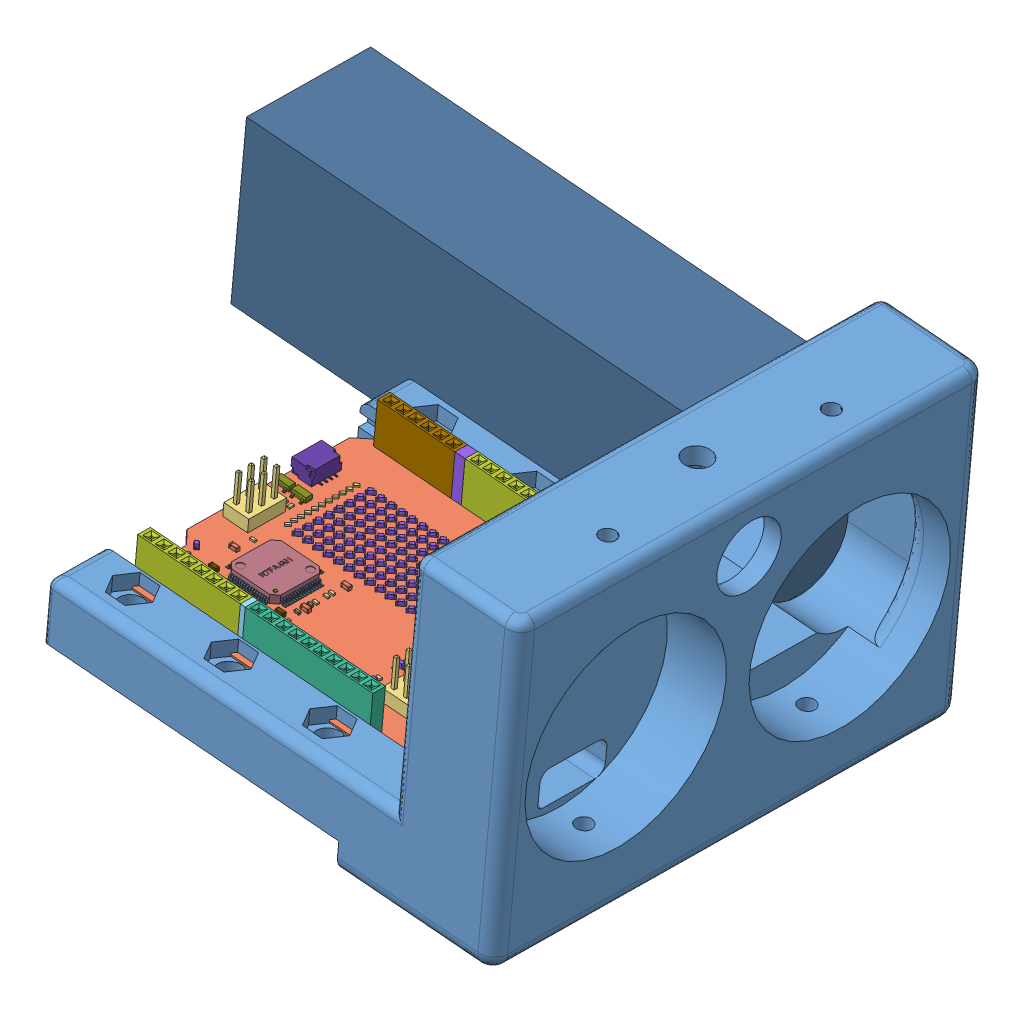
SolidWorks assembly SensorboxController1, configuration Standard. Lengths in mm.
Overall size (130.07 72.74 100.91).
576 component instances, 46 part files, 4 mates.
Components (placement in the parent):
- Sensorbox_small_arduino-1: Sensorbox_small_arduino [Standard] at (44.4865 -57.9317 279.8845) x (0.001937 -0.010295 -0.999945) z (0.996616 -0.082156 0.002776) size (100 64 96.5)
- PCB(ABX00087).step-1: PCB(ABX00087).step [Standard] at (42.9255 -81.7651 134.9822) x (-0.996616 0.082156 -0.002776) z (0.08218 0.996566 -0.010101) size (70.54 53.34 14.5)
  - Board.step-1: Board.step [Standard] at origin size (68.58 53.34 1.61)
    - Open CASCADE STEP translator 7.5 4.1.1.step-1: Open CASCADE STEP translator 7.5 4.1.1.step [Standard] at (0 0 -1.6063) size (68.58 53.34 1.61)
  - R60.step-1: R60.step [Standard] at origin size (1 0.5 0.34)
    - RES-0402.step-1: RES-0402.step [Standard] at (26.4 44.3 0) size (1 0.5 0.34)
  - R59.step-1: R59.step [Standard] at origin size (1 0.5 0.34)
    - RES-0402.step-1: RES-0402.step [Standard] at (26.416 41.021 0) x (-1 0 0) z (0 0 1) size (1 0.5 0.34)
  - R20.step-1: R20.step [Standard] at origin size (1 0.5 0.34)
    - RES-0402.step-1: RES-0402.step [Standard] at (24.29 35.433 0) x (-1 0 0) z (0 0 1) size (1 0.5 0.34)
  - U5.step-1: U5.step [Standard] at origin size (6.71 7 1.8)
    - 6430901664.step-1: 6430901664.step [Standard] at (26.325 10.206 0) x (0 -1 0) z (0 0 1) size (7 6.71 1.8)
      - Body.step-1: Body.step [Standard] at (-1.85 -3.35 0.02) size (3.71 6.71 1.78)
        - Open CASCADE STEP translator 6.8 29.1.1.step-1: Open CASCADE STEP translator 6.8 29.1.1.step [Standard] at origin size (3.71 6.71 1.78)
      - Lead.step-1: Lead.step [Standard] at (-1.85 -2.3 0) x (-1 0 0) z (0 0 1) size (1.65 0.75 1.01)
      - Lead.step-2: Lead.step [Standard] at (-1.85 0 0) x (-1 0 0) z (0 0 1) size (1.65 0.75 1.01)
      - Lead.step-3: Lead.step [Standard] at (-1.85 2.3 0) x (-1 0 0) z (0 0 1) size (1.65 0.75 1.01)
      - Tab.step-1: Tab.step [Standard] at (1.85 0 0) size (1.65 3 1.01)
  - C28.step-1: C28.step [Standard] at origin size (1.25 2 1.25)
    - CAP-0805.step-1: CAP-0805.step [Standard] at (31.0249 12.3561 0) x (0 1 0) z (0 0 1) size (2 1.25 1.25)
  - R58.step-1: R58.step [Standard] at origin size (1 0.5 0.34)
    - RES-0402.step-1: RES-0402.step [Standard] at (16.825 30.966 0) x (-1 0 0) z (0 0 1) size (1 0.5 0.34)
  - R57.step-1: R57.step [Standard] at origin size (1 0.5 0.34)
    - RES-0402.step-1: RES-0402.step [Standard] at (3.625 31.766 0) size (1 0.5 0.34)
  - R16.step-1: R16.step [Standard] at origin size (1.06 1.06 0.34)
    - RES-0402.step-1: RES-0402.step [Standard] at (60.0141 13.5803 0) x (0.707107 0.707107 0) z (0 0 1) size (1 0.5 0.34)
  - R14.step-1: R14.step [Standard] at origin size (1.06 1.06 0.34)
    - RES-0402.step-1: RES-0402.step [Standard] at (60.0141 12.1803 0) x (0.707107 0.707107 0) z (0 0 1) size (1 0.5 0.34)
  - R2.step-1: R2.step [Standard] at origin size (1.06 1.06 0.34)
    - RES-0402.step-1: RES-0402.step [Standard] at (59.9205 26.112 0) x (0.707107 0.707107 0) z (0 0 1) size (1 0.5 0.34)
  - 96.step-1: 96.step [Standard] at origin size (1.7 1.7 0.8)
    - HSMx-190.step-1: HSMx-190.step [Standard] at (57.5124 11.8305 0) x (-0.707107 -0.707107 0) z (0 0 1) size (1.6 0.8 0.8)
  - 95.step-1: 95.step [Standard] at origin size (1.7 1.7 0.8)
    - HSMx-190.step-1: HSMx-190.step [Standard] at (55.4124 11.8305 0) x (-0.707107 -0.707107 0) z (0 0 1) size (1.6 0.8 0.8)
  - 94.step-1: 94.step [Standard] at origin size (1.7 1.7 0.8)
    - HSMx-190.step-1: HSMx-190.step [Standard] at (53.3124 11.8305 0) x (-0.707107 -0.707107 0) z (0 0 1) size (1.6 0.8 0.8)
  - 93.step-1: 93.step [Standard] at origin size (1.7 1.7 0.8)
    - HSMx-190.step-1: HSMx-190.step [Standard] at (51.2124 11.8305 0) x (-0.707107 -0.707107 0) z (0 0 1) size (1.6 0.8 0.8)
  - 92.step-1: 92.step [Standard] at origin size (1.7 1.7 0.8)
    - HSMx-190.step-1: HSMx-190.step [Standard] at (49.1124 11.8305 0) x (-0.707107 -0.707107 0) z (0 0 1) size (1.6 0.8 0.8)
  - 91.step-1: 91.step [Standard] at origin size (1.7 1.7 0.8)
    - HSMx-190.step-1: HSMx-190.step [Standard] at (47.0124 11.8305 0) x (-0.707107 -0.707107 0) z (0 0 1) size (1.6 0.8 0.8)
  - 90.step-1: 90.step [Standard] at origin size (1.7 1.7 0.8)
    - HSMx-190.step-1: HSMx-190.step [Standard] at (44.9124 11.8305 0) x (-0.707107 -0.707107 0) z (0 0 1) size (1.6 0.8 0.8)
  - 89.step-1: 89.step [Standard] at origin size (1.7 1.7 0.8)
    - HSMx-190.step-1: HSMx-190.step [Standard] at (42.8124 11.8305 0) x (-0.707107 -0.707107 0) z (0 0 1) size (1.6 0.8 0.8)
  - 88.step-1: 88.step [Standard] at origin size (1.7 1.7 0.8)
    - HSMx-190.step-1: HSMx-190.step [Standard] at (40.7124 11.8305 0) x (-0.707107 -0.707107 0) z (0 0 1) size (1.6 0.8 0.8)
  - 87.step-1: 87.step [Standard] at origin size (1.7 1.7 0.8)
    - HSMx-190.step-1: HSMx-190.step [Standard] at (38.6124 11.8305 0) x (-0.707107 -0.707107 0) z (0 0 1) size (1.6 0.8 0.8)
  - 86.step-1: 86.step [Standard] at origin size (1.7 1.7 0.8)
    - HSMx-190.step-1: HSMx-190.step [Standard] at (36.5124 11.8305 0) x (-0.707107 -0.707107 0) z (0 0 1) size (1.6 0.8 0.8)
  - 85.step-1: 85.step [Standard] at origin size (1.7 1.7 0.8)
    - HSMx-190.step-1: HSMx-190.step [Standard] at (34.4124 11.8305 0) x (-0.707107 -0.707107 0) z (0 0 1) size (1.6 0.8 0.8)
  - 84.step-1: 84.step [Standard] at origin size (1.7 1.7 0.8)
    - HSMx-190.step-1: HSMx-190.step [Standard] at (57.5124 13.9305 0) x (-0.707107 -0.707107 0) z (0 0 1) size (1.6 0.8 0.8)
  - 83.step-1: 83.step [Standard] at origin size (1.7 1.7 0.8)
    - HSMx-190.step-1: HSMx-190.step [Standard] at (55.4124 13.9305 0) x (-0.707107 -0.707107 0) z (0 0 1) size (1.6 0.8 0.8)
  - 82.step-1: 82.step [Standard] at origin size (1.7 1.7 0.8)
    - HSMx-190.step-1: HSMx-190.step [Standard] at (53.3 13.9182 0) x (-0.707107 -0.707107 0) z (0 0 1) size (1.6 0.8 0.8)
  - 81.step-1: 81.step [Standard] at origin size (1.7 1.7 0.8)
    - HSMx-190.step-1: HSMx-190.step [Standard] at (51.2124 13.9305 0) x (-0.707107 -0.707107 0) z (0 0 1) size (1.6 0.8 0.8)
  - 80.step-1: 80.step [Standard] at origin size (1.7 1.7 0.8)
    - HSMx-190.step-1: HSMx-190.step [Standard] at (49.1124 13.9305 0) x (-0.707107 -0.707107 0) z (0 0 1) size (1.6 0.8 0.8)
  - 79.step-1: 79.step [Standard] at origin size (1.7 1.7 0.8)
    - HSMx-190.step-1: HSMx-190.step [Standard] at (47.0124 13.9305 0) x (-0.707107 -0.707107 0) z (0 0 1) size (1.6 0.8 0.8)
  - 78.step-1: 78.step [Standard] at origin size (1.7 1.7 0.8)
    - HSMx-190.step-1: HSMx-190.step [Standard] at (44.9124 13.9305 0) x (-0.707107 -0.707107 0) z (0 0 1) size (1.6 0.8 0.8)
  - 77.step-1: 77.step [Standard] at origin size (1.7 1.7 0.8)
    - HSMx-190.step-1: HSMx-190.step [Standard] at (42.8124 13.9305 0) x (-0.707107 -0.707107 0) z (0 0 1) size (1.6 0.8 0.8)
  - 76.step-1: 76.step [Standard] at origin size (1.7 1.7 0.8)
    - HSMx-190.step-1: HSMx-190.step [Standard] at (40.7124 13.9305 0) x (-0.707107 -0.707107 0) z (0 0 1) size (1.6 0.8 0.8)
  - 75.step-1: 75.step [Standard] at origin size (1.7 1.7 0.8)
    - HSMx-190.step-1: HSMx-190.step [Standard] at (38.6124 13.9305 0) x (-0.707107 -0.707107 0) z (0 0 1) size (1.6 0.8 0.8)
  - 74.step-1: 74.step [Standard] at origin size (1.7 1.7 0.8)
    - HSMx-190.step-1: HSMx-190.step [Standard] at (36.5124 13.9305 0) x (-0.707107 -0.707107 0) z (0 0 1) size (1.6 0.8 0.8)
  - 73.step-1: 73.step [Standard] at origin size (1.7 1.7 0.8)
    - HSMx-190.step-1: HSMx-190.step [Standard] at (34.4124 13.9305 0) x (-0.707107 -0.707107 0) z (0 0 1) size (1.6 0.8 0.8)
  - 72.step-1: 72.step [Standard] at origin size (1.7 1.7 0.8)
    - HSMx-190.step-1: HSMx-190.step [Standard] at (57.5124 16.0305 0) x (-0.707107 -0.707107 0) z (0 0 1) size (1.6 0.8 0.8)
  - 71.step-1: 71.step [Standard] at origin size (1.7 1.7 0.8)
    - HSMx-190.step-1: HSMx-190.step [Standard] at (55.4124 16.0305 0) x (-0.707107 -0.707107 0) z (0 0 1) size (1.6 0.8 0.8)
  - 70.step-1: 70.step [Standard] at origin size (1.7 1.7 0.8)
    - HSMx-190.step-1: HSMx-190.step [Standard] at (53.3124 16.0305 0) x (-0.707107 -0.707107 0) z (0 0 1) size (1.6 0.8 0.8)
  - 69.step-1: 69.step [Standard] at origin size (1.7 1.7 0.8)
    - HSMx-190.step-1: HSMx-190.step [Standard] at (51.2124 16.0305 0) x (-0.707107 -0.707107 0) z (0 0 1) size (1.6 0.8 0.8)
  - 68.step-1: 68.step [Standard] at origin size (1.7 1.7 0.8)
    - HSMx-190.step-1: HSMx-190.step [Standard] at (49.1124 16.0305 0) x (-0.707107 -0.707107 0) z (0 0 1) size (1.6 0.8 0.8)
  - 67.step-1: 67.step [Standard] at origin size (1.7 1.7 0.8)
    - HSMx-190.step-1: HSMx-190.step [Standard] at (47.0124 16.0305 0) x (-0.707107 -0.707107 0) z (0 0 1) size (1.6 0.8 0.8)
  - 66.step-1: 66.step [Standard] at origin size (1.7 1.7 0.8)
    - HSMx-190.step-1: HSMx-190.step [Standard] at (44.9124 16.0305 0) x (-0.707107 -0.707107 0) z (0 0 1) size (1.6 0.8 0.8)
  - 65.step-1: 65.step [Standard] at origin size (1.7 1.7 0.8)
    - HSMx-190.step-1: HSMx-190.step [Standard] at (42.8124 16.0305 0) x (-0.707107 -0.707107 0) z (0 0 1) size (1.6 0.8 0.8)
  - 64.step-1: 64.step [Standard] at origin size (1.7 1.7 0.8)
    - HSMx-190.step-1: HSMx-190.step [Standard] at (40.7124 16.0305 0) x (-0.707107 -0.707107 0) z (0 0 1) size (1.6 0.8 0.8)
  - 63.step-1: 63.step [Standard] at origin size (1.7 1.7 0.8)
    - HSMx-190.step-1: HSMx-190.step [Standard] at (38.6124 16.0305 0) x (-0.707107 -0.707107 0) z (0 0 1) size (1.6 0.8 0.8)
  - 62.step-1: 62.step [Standard] at origin size (1.7 1.7 0.8)
    - HSMx-190.step-1: HSMx-190.step [Standard] at (36.5124 16.0305 0) x (-0.707107 -0.707107 0) z (0 0 1) size (1.6 0.8 0.8)
  - 61.step-1: 61.step [Standard] at origin size (1.7 1.7 0.8)
    - HSMx-190.step-1: HSMx-190.step [Standard] at (34.412 16.0302 0) x (-0.707107 -0.707107 0) z (0 0 1) size (1.6 0.8 0.8)
  - 60.step-1: 60.step [Standard] at origin size (1.7 1.7 0.8)
    - HSMx-190.step-1: HSMx-190.step [Standard] at (57.5124 18.1305 0) x (-0.707107 -0.707107 0) z (0 0 1) size (1.6 0.8 0.8)
  - 59.step-1: 59.step [Standard] at origin size (1.7 1.7 0.8)
    - HSMx-190.step-1: HSMx-190.step [Standard] at (55.4124 18.1305 0) x (-0.707107 -0.707107 0) z (0 0 1) size (1.6 0.8 0.8)
  - 58.step-1: 58.step [Standard] at origin size (1.7 1.7 0.8)
    - HSMx-190.step-1: HSMx-190.step [Standard] at (53.3124 18.1305 0) x (-0.707107 -0.707107 0) z (0 0 1) size (1.6 0.8 0.8)
  - 57.step-1: 57.step [Standard] at origin size (1.7 1.7 0.8)
    - HSMx-190.step-1: HSMx-190.step [Standard] at (51.2124 18.1305 0) x (-0.707107 -0.707107 0) z (0 0 1) size (1.6 0.8 0.8)
  - 56.step-1: 56.step [Standard] at origin size (1.7 1.7 0.8)
    - HSMx-190.step-1: HSMx-190.step [Standard] at (49.1124 18.1305 0) x (-0.707107 -0.707107 0) z (0 0 1) size (1.6 0.8 0.8)
  - U6.step-1: U6.step [Standard] at origin size (2.1 2.21 1.1)
    - 6430901184.step-1: 6430901184.step [Standard] at (12.525 36.466 0) x (-1 0 0) z (0 0 1) size (2.1 2.21 1.1)
      - Body-1.step-1: Body-1.step [Standard] at (-0.7 -1.1 0) size (1.41 2.21 1.1)
        - Open CASCADE STEP translator 7.5 28.2.1.step-1: Open CASCADE STEP translator 7.5 28.2.1.step [Standard] at origin size (1.41 2.21 1.1)
      - Open CASCADE STEP translator 7.5 28.1.step-1: Open CASCADE STEP translator 7.5 28.1.step [Standard] at (-0.7 -1.1 0.001) size (0.18 0.18 0)
      - Leader.step-1: Leader.step [Standard] at (-0.7 -0.65 0) x (-1 0 0) z (0 0 1) size (0.37 0.2 0.6)
      - Leader.step-2: Leader.step [Standard] at (-0.7 0 0) x (-1 0 0) z (0 0 1) size (0.37 0.2 0.6)
      - Leader.step-3: Leader.step [Standard] at (-0.7 0.65 0) x (-1 0 0) z (0 0 1) size (0.37 0.2 0.6)
      - Leader.step-4: Leader.step [Standard] at (0.7 -0.65 0) size (0.37 0.2 0.6)
      - Leader.step-5: Leader.step [Standard] at (0.7 0 0) size (0.37 0.2 0.6)
      - Leader.step-6: Leader.step [Standard] at (0.7 0.65 0) size (0.37 0.2 0.6)
  - U2.step-1: U2.step [Standard] at origin size (2.1 2.21 1.1)
    - 6430901184.step-1: 6430901184.step [Standard] at (12.525 39.266 0) x (-1 0 0) z (0 0 1) size (2.1 2.21 1.1)
      - Body-1.step-1: Body-1.step [Standard] at (-0.7 -1.1 0) size (1.41 2.21 1.1)
        - Open CASCADE STEP translator 7.5 28.2.1.step-1: Open CASCADE STEP translator 7.5 28.2.1.step [Standard] at origin size (1.41 2.21 1.1)
      - Open CASCADE STEP translator 7.5 28.1.step-1: Open CASCADE STEP translator 7.5 28.1.step [Standard] at (-0.7 -1.1 0.001) size (0.18 0.18 0)
      - Leader.step-1: Leader.step [Standard] at (-0.7 -0.65 0) x (-1 0 0) z (0 0 1) size (0.37 0.2 0.6)
      - Leader.step-2: Leader.step [Standard] at (-0.7 0 0) x (-1 0 0) z (0 0 1) size (0.37 0.2 0.6)
      - Leader.step-3: Leader.step [Standard] at (-0.7 0.65 0) x (-1 0 0) z (0 0 1) size (0.37 0.2 0.6)
      - Leader.step-4: Leader.step [Standard] at (0.7 -0.65 0) size (0.37 0.2 0.6)
      - Leader.step-5: Leader.step [Standard] at (0.7 0 0) size (0.37 0.2 0.6)
      - Leader.step-6: Leader.step [Standard] at (0.7 0.65 0) size (0.37 0.2 0.6)
  - C30.step-1: C30.step [Standard] at origin size (1 0.5 0.5)
    - CAP-0402.step-1: CAP-0402.step [Standard] at (12.525 41.266 0) x (-1 0 0) z (0 0 1) size (1 0.5 0.5)
  - C29.step-1: C29.step [Standard] at origin size (0.5 1 0.5)
    - CAP-0402.step-1: CAP-0402.step [Standard] at (11.925 34.231 0) x (0 1 0) z (0 0 1) size (1 0.5 0.5)
  - R3.step-1: R3.step [Standard] at origin size (0.5 1 0.34)
    - RES-0402.step-1: RES-0402.step [Standard] at (13.466 47.244 0) x (0 -1 0) z (0 0 1) size (1 0.5 0.34)
  - M1.step-1: M1.step [Standard] at origin size (20.65 15.55 2.45)
    - 6428909520.step-1: 6428909520.step [Standard] at (13.625 21.5 0.05) size (13.55 14.15 2.45)
      - Extruded.step-1: Extruded.step [Standard] at origin size (13.55 14.15 2.45)
    - 6428905200.step-1: 6428905200.step [Standard] at (10.575 21.5 0.05) size (20.65 15.55 0.8)
      - Extruded-0.step-1: Extruded-0.step [Standard] at origin size (20.65 15.55 0.8)
  - F1.step-1: F1.step [Standard] at origin size (3.4 4.8 1.4)
    - 6431039776.step-1: 6431039776.step [Standard] at (9.125 32.603 0) size (3.4 4.8 1.4)
      - Extruded-1.step-1: Extruded-1.step [Standard] at origin size (3.4 4.8 1.4)
  - R52.step-1: R52.step [Standard] at origin size (1 0.5 0.34)
    - RES-0402.step-1: RES-0402.step [Standard] at (9.125 42.8599 0) size (1 0.5 0.34)
  - R26.step-1: R26.step [Standard] at origin size (1 0.5 0.34)
    - RES-0402.step-1: RES-0402.step [Standard] at (6.025 30.666 0) x (-1 0 0) z (0 0 1) size (1 0.5 0.34)
  - R12.step-1: R12.step [Standard] at origin size (0.5 1 0.34)
    - RES-0402.step-1: RES-0402.step [Standard] at (67.2698 22.8345 0) x (0 -1 0) z (0 0 1) size (1 0.5 0.34)
  - R11.step-1: R11.step [Standard] at origin size (0.5 1 0.34)
    - RES-0402.step-1: RES-0402.step [Standard] at (66.0698 22.8345 0) x (0 -1 0) z (0 0 1) size (1 0.5 0.34)
  - R10.step-1: R10.step [Standard] at origin size (0.5 1 0.34)
    - RES-0402.step-1: RES-0402.step [Standard] at (63.8698 22.8345 0) x (0 -1 0) z (0 0 1) size (1 0.5 0.34)
  - R9.step-1: R9.step [Standard] at origin size (0.5 1 0.34)
    - RES-0402.step-1: RES-0402.step [Standard] at (62.6698 22.8345 0) x (0 -1 0) z (0 0 1) size (1 0.5 0.34)
  - Q2.step-1: Q2.step [Standard] at origin size (3 2.5 1.1)
    - SOT-23.step-1: SOT-23.step [Standard] at (66.6698 20.0344 0.55) x (1 0 0) z (0 -1 0) size (3 1.1 2.5)
  - Q1.step-1: Q1.step [Standard] at origin size (3 2.5 1.1)
    - SOT-23.step-1: SOT-23.step [Standard] at (63.2698 20.0344 0.55) x (1 0 0) z (0 -1 0) size (3 1.1 2.5)
  - J2.step-1: J2.step [Standard] at origin size (4.95 6 2.96)
    - SM04B-SRSS-TB_RGB12040119.step-1: SM04B-SRSS-TB_RGB12040119.step [Standard] at (64.3195 14.346 -0.28) x (0 1 0) z (1 0 0) size (6 2.96 4.95)
  - R13.step-1: R13.step [Standard] at origin size (1 0.5 0.34)
    - RES-0402.step-1: RES-0402.step [Standard] at (44.646 35.676 0) x (-1 0 0) z (0 0 1) size (1 0.5 0.34)
  - R47.step-1: R47.step [Standard] at origin size (0.5 1 0.34)
    - RES-0402.step-1: RES-0402.step [Standard] at (20.346 36.576 0) x (0 -1 0) z (0 0 1) size (1 0.5 0.34)
  - R48.step-1: R48.step [Standard] at origin size (0.5 1 0.34)
    - RES-0402.step-1: RES-0402.step [Standard] at (21.446 36.576 0) x (0 -1 0) z (0 0 1) size (1 0.5 0.34)
  - R46.step-1: R46.step [Standard] at origin size (0.5 1 0.34)
    - RES-0402.step-1: RES-0402.step [Standard] at (15.946 36.576 0) x (0 -1 0) z (0 0 1) size (1 0.5 0.34)
  - R45.step-1: R45.step [Standard] at origin size (0.5 1 0.34)
    - RES-0402.step-1: RES-0402.step [Standard] at (17.046 36.576 0) x (0 -1 0) z (0 0 1) size (1 0.5 0.34)
  - R31.step-1: R31.step [Standard] at origin size (1.06 1.06 0.34)
    - RES-0402.step-1: RES-0402.step [Standard] at (60.0141 20.5803 0) x (0.707107 0.707107 0) z (0 0 1) size (1 0.5 0.34)
  - 42.step-1: 42.step [Standard] at origin size (1.7 1.7 0.8)
    - HSMx-190.step-1: HSMx-190.step [Standard] at (44.9124 20.2305 0) x (-0.707107 -0.707107 0) z (0 0 1) size (1.6 0.8 0.8)
  - R34.step-1: R34.step [Standard] at origin size (1.06 1.06 0.34)
    - RES-0402.step-1: RES-0402.step [Standard] at (60.0141 24.7803 0) x (0.707107 0.707107 0) z (0 0 1) size (1 0.5 0.34)
  - R33.step-1: R33.step [Standard] at origin size (1.06 1.06 0.34)
    - RES-0402.step-1: RES-0402.step [Standard] at (60.0141 23.3803 0) x (0.707107 0.707107 0) z (0 0 1) size (1 0.5 0.34)
  - R32.step-1: R32.step [Standard] at origin size (1.06 1.06 0.34)
    - RES-0402.step-1: RES-0402.step [Standard] at (60.0141 21.9803 0) x (0.707107 0.707107 0) z (0 0 1) size (1 0.5 0.34)
  - R30.step-1: R30.step [Standard] at origin size (1.06 1.06 0.34)
    - RES-0402.step-1: RES-0402.step [Standard] at (60.0141 19.1803 0) x (0.707107 0.707107 0) z (0 0 1) size (1 0.5 0.34)
  - R29.step-1: R29.step [Standard] at origin size (1.06 1.06 0.34)
    - RES-0402.step-1: RES-0402.step [Standard] at (60.0141 17.7803 0) x (0.707107 0.707107 0) z (0 0 1) size (1 0.5 0.34)
  - R28.step-1: R28.step [Standard] at origin size (1.06 1.06 0.34)
    - RES-0402.step-1: RES-0402.step [Standard] at (60.0141 16.3803 0) x (0.707107 0.707107 0) z (0 0 1) size (1 0.5 0.34)
  - R27.step-1: R27.step [Standard] at origin size (1.06 1.06 0.34)
    - RES-0402.step-1: RES-0402.step [Standard] at (60.0141 14.9803 0) x (0.707107 0.707107 0) z (0 0 1) size (1 0.5 0.34)
  - 54.step-1: 54.step [Standard] at origin size (1.7 1.7 0.8)
    - HSMx-190.step-1: HSMx-190.step [Standard] at (44.9124 18.1305 0) x (-0.707107 -0.707107 0) z (0 0 1) size (1.6 0.8 0.8)
  - 52.step-1: 52.step [Standard] at origin size (1.7 1.7 0.8)
    - HSMx-190.step-1: HSMx-190.step [Standard] at (40.7124 18.1305 0) x (-0.707107 -0.707107 0) z (0 0 1) size (1.6 0.8 0.8)
  - 50.step-1: 50.step [Standard] at origin size (1.7 1.7 0.8)
    - HSMx-190.step-1: HSMx-190.step [Standard] at (36.5124 18.1305 0) x (-0.707107 -0.707107 0) z (0 0 1) size (1.6 0.8 0.8)
  - 48.step-1: 48.step [Standard] at origin size (1.7 1.7 0.8)
    - HSMx-190.step-1: HSMx-190.step [Standard] at (57.5124 20.2305 0) x (-0.707107 -0.707107 0) z (0 0 1) size (1.6 0.8 0.8)
  - 46.step-1: 46.step [Standard] at origin size (1.7 1.7 0.8)
    - HSMx-190.step-1: HSMx-190.step [Standard] at (53.3124 20.2305 0) x (-0.707107 -0.707107 0) z (0 0 1) size (1.6 0.8 0.8)
  - 44.step-1: 44.step [Standard] at origin size (1.7 1.7 0.8)
    - HSMx-190.step-1: HSMx-190.step [Standard] at (49.1124 20.2305 0) x (-0.707107 -0.707107 0) z (0 0 1) size (1.6 0.8 0.8)
  - 55.step-1: 55.step [Standard] at origin size (1.7 1.7 0.8)
    - HSMx-190.step-1: HSMx-190.step [Standard] at (47.0124 18.1305 0) x (-0.707107 -0.707107 0) z (0 0 1) size (1.6 0.8 0.8)
  - 53.step-1: 53.step [Standard] at origin size (1.7 1.7 0.8)
    - HSMx-190.step-1: HSMx-190.step [Standard] at (42.8124 18.1305 0) x (-0.707107 -0.707107 0) z (0 0 1) size (1.6 0.8 0.8)
  - 51.step-1: 51.step [Standard] at origin size (1.7 1.7 0.8)
    - HSMx-190.step-1: HSMx-190.step [Standard] at (38.6124 18.1305 0) x (-0.707107 -0.707107 0) z (0 0 1) size (1.6 0.8 0.8)
  - 49.step-1: 49.step [Standard] at origin size (1.7 1.7 0.8)
    - HSMx-190.step-1: HSMx-190.step [Standard] at (34.4124 18.1305 0) x (-0.707107 -0.707107 0) z (0 0 1) size (1.6 0.8 0.8)
  - 47.step-1: 47.step [Standard] at origin size (1.7 1.7 0.8)
    - HSMx-190.step-1: HSMx-190.step [Standard] at (55.4124 20.2305 0) x (-0.707107 -0.707107 0) z (0 0 1) size (1.6 0.8 0.8)
  - 45.step-1: 45.step [Standard] at origin size (1.7 1.7 0.8)
    - HSMx-190.step-1: HSMx-190.step [Standard] at (51.2124 20.2305 0) x (-0.707107 -0.707107 0) z (0 0 1) size (1.6 0.8 0.8)
  - 43.step-1: 43.step [Standard] at origin size (1.7 1.7 0.8)
    - HSMx-190.step-1: HSMx-190.step [Standard] at (47.0124 20.2305 0) x (-0.707107 -0.707107 0) z (0 0 1) size (1.6 0.8 0.8)
  - 40.step-1: 40.step [Standard] at origin size (1.7 1.7 0.8)
    - HSMx-190.step-1: HSMx-190.step [Standard] at (40.7124 20.2305 0) x (-0.707107 -0.707107 0) z (0 0 1) size (1.6 0.8 0.8)
  - 38.step-1: 38.step [Standard] at origin size (1.7 1.7 0.8)
    - HSMx-190.step-1: HSMx-190.step [Standard] at (36.5124 20.2305 0) x (-0.707107 -0.707107 0) z (0 0 1) size (1.6 0.8 0.8)
  - 36.step-1: 36.step [Standard] at origin size (1.7 1.7 0.8)
    - HSMx-190.step-1: HSMx-190.step [Standard] at (57.5124 22.3305 0) x (-0.707107 -0.707107 0) z (0 0 1) size (1.6 0.8 0.8)
  - 34.step-1: 34.step [Standard] at origin size (1.7 1.7 0.8)
    - HSMx-190.step-1: HSMx-190.step [Standard] at (53.3124 22.3305 0) x (-0.707107 -0.707107 0) z (0 0 1) size (1.6 0.8 0.8)
  - 32.step-1: 32.step [Standard] at origin size (1.7 1.7 0.8)
    - HSMx-190.step-1: HSMx-190.step [Standard] at (49.1124 22.3305 0) x (-0.707107 -0.707107 0) z (0 0 1) size (1.6 0.8 0.8)
  - 41.step-1: 41.step [Standard] at origin size (1.7 1.7 0.8)
    - HSMx-190.step-1: HSMx-190.step [Standard] at (42.8124 20.2305 0) x (-0.707107 -0.707107 0) z (0 0 1) size (1.6 0.8 0.8)
  - 39.step-1: 39.step [Standard] at origin size (1.7 1.7 0.8)
    - HSMx-190.step-1: HSMx-190.step [Standard] at (38.6124 20.2305 0) x (-0.707107 -0.707107 0) z (0 0 1) size (1.6 0.8 0.8)
  - 37.step-1: 37.step [Standard] at origin size (1.7 1.7 0.8)
    - HSMx-190.step-1: HSMx-190.step [Standard] at (34.4124 20.2305 0) x (-0.707107 -0.707107 0) z (0 0 1) size (1.6 0.8 0.8)
  - 35.step-1: 35.step [Standard] at origin size (1.7 1.7 0.8)
    - HSMx-190.step-1: HSMx-190.step [Standard] at (55.4124 22.3305 0) x (-0.707107 -0.707107 0) z (0 0 1) size (1.6 0.8 0.8)
  - 33.step-1: 33.step [Standard] at origin size (1.7 1.7 0.8)
    - HSMx-190.step-1: HSMx-190.step [Standard] at (51.2124 22.3305 0) x (-0.707107 -0.707107 0) z (0 0 1) size (1.6 0.8 0.8)
  - 31.step-1: 31.step [Standard] at origin size (1.7 1.7 0.8)
    - HSMx-190.step-1: HSMx-190.step [Standard] at (47.0124 22.3305 0) x (-0.707107 -0.707107 0) z (0 0 1) size (1.6 0.8 0.8)
  - 30.step-1: 30.step [Standard] at origin size (1.7 1.7 0.8)
    - HSMx-190.step-1: HSMx-190.step [Standard] at (44.9124 22.3305 0) x (-0.707107 -0.707107 0) z (0 0 1) size (1.6 0.8 0.8)
  - 28.step-1: 28.step [Standard] at origin size (1.7 1.7 0.8)
    - HSMx-190.step-1: HSMx-190.step [Standard] at (40.7124 22.3305 0) x (-0.707107 -0.707107 0) z (0 0 1) size (1.6 0.8 0.8)
  - 26.step-1: 26.step [Standard] at origin size (1.7 1.7 0.8)
    - HSMx-190.step-1: HSMx-190.step [Standard] at (36.5124 22.3305 0) x (-0.707107 -0.707107 0) z (0 0 1) size (1.6 0.8 0.8)
  - 24.step-1: 24.step [Standard] at origin size (1.7 1.7 0.8)
    - HSMx-190.step-1: HSMx-190.step [Standard] at (57.5124 24.4305 0) x (-0.707107 -0.707107 0) z (0 0 1) size (1.6 0.8 0.8)
  - 22.step-1: 22.step [Standard] at origin size (1.7 1.7 0.8)
    - HSMx-190.step-1: HSMx-190.step [Standard] at (53.3124 24.4305 0) x (-0.707107 -0.707107 0) z (0 0 1) size (1.6 0.8 0.8)
  - 29.step-1: 29.step [Standard] at origin size (1.7 1.7 0.8)
    - HSMx-190.step-1: HSMx-190.step [Standard] at (42.8124 22.3305 0) x (-0.707107 -0.707107 0) z (0 0 1) size (1.6 0.8 0.8)
  - 27.step-1: 27.step [Standard] at origin size (1.7 1.7 0.8)
    - HSMx-190.step-1: HSMx-190.step [Standard] at (38.6124 22.3305 0) x (-0.707107 -0.707107 0) z (0 0 1) size (1.6 0.8 0.8)
  - 25.step-1: 25.step [Standard] at origin size (1.7 1.7 0.8)
    - HSMx-190.step-1: HSMx-190.step [Standard] at (34.4124 22.3305 0) x (-0.707107 -0.707107 0) z (0 0 1) size (1.6 0.8 0.8)
  - 23.step-1: 23.step [Standard] at origin size (1.7 1.7 0.8)
    - HSMx-190.step-1: HSMx-190.step [Standard] at (55.4124 24.4305 0) x (-0.707107 -0.707107 0) z (0 0 1) size (1.6 0.8 0.8)
  - 21.step-1: 21.step [Standard] at origin size (1.7 1.7 0.8)
    - HSMx-190.step-1: HSMx-190.step [Standard] at (51.2124 24.4305 0) x (-0.707107 -0.707107 0) z (0 0 1) size (1.6 0.8 0.8)
  - 20.step-1: 20.step [Standard] at origin size (1.7 1.7 0.8)
    - HSMx-190.step-1: HSMx-190.step [Standard] at (49.1124 24.4305 0) x (-0.707107 -0.707107 0) z (0 0 1) size (1.6 0.8 0.8)
  - 18.step-1: 18.step [Standard] at origin size (1.7 1.7 0.8)
    - HSMx-190.step-1: HSMx-190.step [Standard] at (44.9124 24.4305 0) x (-0.707107 -0.707107 0) z (0 0 1) size (1.6 0.8 0.8)
  - 16.step-1: 16.step [Standard] at origin size (1.7 1.7 0.8)
    - HSMx-190.step-1: HSMx-190.step [Standard] at (40.7124 24.4305 0) x (-0.707107 -0.707107 0) z (0 0 1) size (1.6 0.8 0.8)
  - 14.step-1: 14.step [Standard] at origin size (1.7 1.7 0.8)
    - HSMx-190.step-1: HSMx-190.step [Standard] at (36.5124 24.4305 0) x (-0.707107 -0.707107 0) z (0 0 1) size (1.6 0.8 0.8)
  - 19.step-1: 19.step [Standard] at origin size (1.7 1.7 0.8)
    - HSMx-190.step-1: HSMx-190.step [Standard] at (47.0124 24.4305 0) x (-0.707107 -0.707107 0) z (0 0 1) size (1.6 0.8 0.8)
  - 17.step-1: 17.step [Standard] at origin size (1.7 1.7 0.8)
    - HSMx-190.step-1: HSMx-190.step [Standard] at (42.8124 24.4305 0) x (-0.707107 -0.707107 0) z (0 0 1) size (1.6 0.8 0.8)
  - 15.step-1: 15.step [Standard] at origin size (1.7 1.7 0.8)
    - HSMx-190.step-1: HSMx-190.step [Standard] at (38.6124 24.4305 0) x (-0.707107 -0.707107 0) z (0 0 1) size (1.6 0.8 0.8)
  - 13.step-1: 13.step [Standard] at origin size (1.7 1.7 0.8)
    - HSMx-190.step-1: HSMx-190.step [Standard] at (34.4124 24.4305 0) x (-0.707107 -0.707107 0) z (0 0 1) size (1.6 0.8 0.8)
  - 12.step-1: 12.step [Standard] at origin size (1.7 1.7 0.8)
    - HSMx-190.step-1: HSMx-190.step [Standard] at (57.5124 26.5305 0) x (-0.707107 -0.707107 0) z (0 0 1) size (1.6 0.8 0.8)
  - 10.step-1: 10.step [Standard] at origin size (1.7 1.7 0.8)
    - HSMx-190.step-1: HSMx-190.step [Standard] at (53.3124 26.5305 0) x (-0.707107 -0.707107 0) z (0 0 1) size (1.6 0.8 0.8)
  - 8.step-1: 8.step [Standard] at origin size (1.7 1.7 0.8)
    - HSMx-190.step-1: HSMx-190.step [Standard] at (49.1124 26.5305 0) x (-0.707107 -0.707107 0) z (0 0 1) size (1.6 0.8 0.8)
  - 11.step-1: 11.step [Standard] at origin size (1.7 1.7 0.8)
    - HSMx-190.step-1: HSMx-190.step [Standard] at (55.4124 26.5305 0) x (-0.707107 -0.707107 0) z (0 0 1) size (1.6 0.8 0.8)
  - 9.step-1: 9.step [Standard] at origin size (1.7 1.7 0.8)
    - HSMx-190.step-1: HSMx-190.step [Standard] at (51.2124 26.5305 0) x (-0.707107 -0.707107 0) z (0 0 1) size (1.6 0.8 0.8)
  - 7.step-1: 7.step [Standard] at origin size (1.7 1.7 0.8)
    - HSMx-190.step-1: HSMx-190.step [Standard] at (47.0124 26.5305 0) x (-0.707107 -0.707107 0) z (0 0 1) size (1.6 0.8 0.8)
  - 6.step-1: 6.step [Standard] at origin size (1.7 1.7 0.8)
    - HSMx-190.step-1: HSMx-190.step [Standard] at (44.9124 26.5305 0) x (-0.707107 -0.707107 0) z (0 0 1) size (1.6 0.8 0.8)
  - 4.step-1: 4.step [Standard] at origin size (1.7 1.7 0.8)
    - HSMx-190.step-1: HSMx-190.step [Standard] at (40.7124 26.5305 0) x (-0.707107 -0.707107 0) z (0 0 1) size (1.6 0.8 0.8)
  - 5.step-1: 5.step [Standard] at origin size (1.7 1.7 0.8)
    - HSMx-190.step-1: HSMx-190.step [Standard] at (42.8124 26.5305 0) x (-0.707107 -0.707107 0) z (0 0 1) size (1.6 0.8 0.8)
  - 3.step-1: 3.step [Standard] at origin size (1.7 1.7 0.8)
    - HSMx-190.step-1: HSMx-190.step [Standard] at (38.6124 26.5305 0) x (-0.707107 -0.707107 0) z (0 0 1) size (1.6 0.8 0.8)
  - 2.step-1: 2.step [Standard] at origin size (1.7 1.7 0.8)
    - HSMx-190.step-1: HSMx-190.step [Standard] at (36.5124 26.5305 0) x (-0.707107 -0.707107 0) z (0 0 1) size (1.6 0.8 0.8)
  - 1.step-1: 1.step [Standard] at origin size (1.7 1.7 0.8)
    - HSMx-190.step-1: HSMx-190.step [Standard] at (34.4124 26.5305 0) x (-0.707107 -0.707107 0) z (0 0 1) size (1.6 0.8 0.8)
  - R35.step-1: R35.step [Standard] at origin size (0.5 1 0.34)
    - RES-0402.step-1: RES-0402.step [Standard] at (22.925 20.8 0) x (0 1 0) z (0 0 1) size (1 0.5 0.34)
  - Q3.step-1: Q3.step [Standard] at origin size (3 2.5 1.1)
    - SOT-23.step-1: SOT-23.step [Standard] at (12.5251 44.0661 0.55) x (-1 0 0) z (0 1 0) size (3 1.1 2.5)
  - D1.step-1: D1.step [Standard] at origin size (2.01 3.7 1.2)
    - SOD123FL.step-1: SOD123FL.step [Standard] at (13.395 12.306 0) x (0 -1 0) z (0 0 1) size (3.7 2 1.2)
      - 8279795424.step-1: 8279795424.step [Standard] at (4 2 0) size (3.7 2 1.2)
        - Body-2.step-1: Body-2.step [Standard] at (-1.5 -1 0) size (3 2 1.2)
          - Open CASCADE STEP translator 7.5 15.1.1.step-1: Open CASCADE STEP translator 7.5 15.1.1.step [Standard] at origin size (3 2 1.2)
        - Lead.step-1: Lead.step [Standard] at (-1.85 -0.425 0) size (1.65 0.75 1.01)
        - Lead.step-2: Lead.step [Standard] at (1.85 0.425 0) x (-1 0 0) z (0 0 1) size (1.65 0.75 1.01)
  - R42.step-1: R42.step [Standard] at origin size (0.5 1 0.34)
    - RES-0402.step-1: RES-0402.step [Standard] at (24.025 23 0) x (0 -1 0) z (0 0 1) size (1 0.5 0.34)
  - R6.step-1: R6.step [Standard] at origin size (0.5 1 0.34)
    - RES-0402.step-1: RES-0402.step [Standard] at (44.1148 41.903 0) x (0 -1 0) z (0 0 1) size (1 0.5 0.34)
  - JOFF.step-1: JOFF.step [Standard] at origin size (7.62 2.54 12.7)
    - pin4.step-1: pin4.step [Standard] at (22.86 2.54 0) size (2.54 2.54 12.7)
    - pin4.step-2: pin4.step [Standard] at (20.32 2.54 0) size (2.54 2.54 12.7)
    - pin4.step-3: pin4.step [Standard] at (17.78 2.54 0) size (2.54 2.54 12.7)
  - C5.step-1: C5.step [Standard] at origin size (1.6 0.8 0.8)
    - CAP-0603.step-1: CAP-0603.step [Standard] at (44.246 29.876 0) size (1.6 0.8 0.8)
  - C18.step-1: C18.step [Standard] at origin size (2 1.25 1.25)
    - CAP-0805.step-1: CAP-0805.step [Standard] at (30.6449 27.1464 0) x (-1 0 0) z (0 0 1) size (2 1.25 1.25)
  - C17.step-1: C17.step [Standard] at origin size (2 1.25 1.25)
    - CAP-0805.step-1: CAP-0805.step [Standard] at (30.6449 25.1964 0) x (-1 0 0) z (0 0 1) size (2 1.25 1.25)
  - J6.step-1: J6.step [Standard] at origin size (7.62 5.04 11.5)
    - 2x3 Header.step-1: 2x3 Header.step [Standard] at (14.9861 39.4239 0) x (0 1 0) z (1 0 0) size (5.04 11.5 7.62)
  - C10.step-1: C10.step [Standard] at origin size (1.25 2 1.25)
    - CAP-0805.step-1: CAP-0805.step [Standard] at (17.5899 10.4061 0) x (0 1 0) z (0 0 1) size (2 1.25 1.25)
  - U4.step-1: U4.step [Standard] at origin size (4 2 0.55)
    - IC_Texas_Instruments_TXB0108DQSR_eec.step-1: IC_Texas_Instruments_TXB0108DQSR_eec.step [Standard] at (13.565 34.6878 0.3) x (1 0 0) z (0 0 1) size (4 2 0.55)
      - Part15.step-1: Part15.step [Standard] at (5.131 -1.3893 -0.25) size (4 2 0.5)
      - Part16.step-1: Part16.step [Standard] at (3.731 -2.1143 -0.3) size (0.2 0.55 0.1)
      - Part16.step-2: Part16.step [Standard] at (4.131 -2.1143 -0.3) size (0.2 0.55 0.1)
      - Part16.step-3: Part16.step [Standard] at (4.531 -2.1143 -0.3) size (0.2 0.55 0.1)
      - Part16.step-4: Part16.step [Standard] at (4.931 -2.1143 -0.3) size (0.2 0.55 0.1)
      - Part16.step-5: Part16.step [Standard] at (5.331 -2.1143 -0.3) size (0.2 0.55 0.1)
      - Part16.step-6: Part16.step [Standard] at (5.731 -2.1143 -0.3) size (0.2 0.55 0.1)
      - Part16.step-7: Part16.step [Standard] at (6.131 -2.1143 -0.3) size (0.2 0.55 0.1)
      - Part16.step-8: Part16.step [Standard] at (6.531 -2.1143 -0.3) size (0.2 0.55 0.1)
      - Part16.step-9: Part16.step [Standard] at (6.931 -2.1143 -0.3) size (0.2 0.55 0.1)
      - Part16_MIR.step-1: Part16_MIR.step [Standard] at (3.731 -0.6643 -0.3) x (1 0 0) z (0 0 -1) size (0.2 0.55 0.1)
